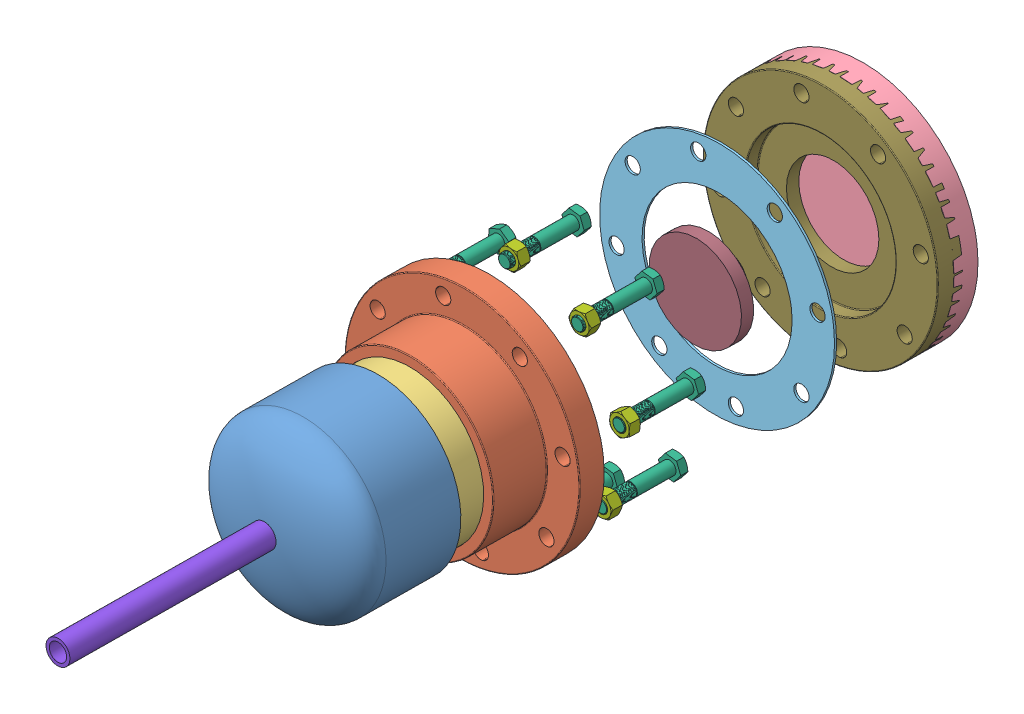
SolidWorks assembly Photogrametry_V4-PVC, configuration Default. Lengths in mm.
Overall size (408.7 414.98 1168.21).
29 component instances, 13 part files, 35 mates.
Components (placement in the parent):
- 8in PVC Cap-1: 8in PVC Cap [4881K523] at (-2621.5848 1342.0566 1037.7149) x (0.006396 0.016238 0.999848) z (-0.99998 0.000109 0.006395) size (216.92 247.14 247.14)
- 8in PVC Flange-1: 8in PVC Flange [4881K224] at (-2623.693 1336.7047 708.1733) x (0.979757 0.199965 -0.009515) z (0.006396 0.016238 0.999848) size (342.9 342.9 115.89)
- 8in PVC Pipe-1: 8in PVC Pipe [48855K43] at (-2622.9517 1338.5865 824.0432) x (0.99998 -0.000109 -0.006395) z (0.006396 0.016238 0.999848) size (219.07 219.07 203.2)
- 8in PVC Flange Closed-1: 8in PVC Flange Closed [4881K973] at (-2627.2283 1327.7296 155.5372) x (0.979757 0.199965 -0.009515) z (0.006396 0.016238 0.999848) size (342.9 342.9 36.51) (hidden)
- 8in Buna-N Gasket-1: 8in Buna-N Gasket [8516T54] at (-2625.8814 1331.149 366.0854) x (0.979757 0.199965 -0.009515) z (0.006396 0.016238 0.999848) size (342.9 342.9 3.17)
- BOLT 3-4in x 4in-1: BOLT 3-4in x 4in [92198A390] at (-2478.1489 1364.8686 603.567) x (0.006396 0.016238 0.999848) z (-0.923711 -0.382898 0.012128) size (114.21 33 28.57)
- BOLT 3-4in x 4in-2: BOLT 3-4in x 4in [92198A390] at (-2542.0965 1459.4699 600.4986) x (0.006396 0.016238 0.999848) z (-0.923711 -0.382898 0.012128) size (114.21 33 28.57)
- BOLT 3-4in x 4in-3: BOLT 3-4in x 4in [92198A390] at (-2499.8414 1252.7986 608.1398) x (0.006396 0.016238 0.999848) z (-0.923711 -0.382898 0.012128) size (114.21 33 28.57)
- BOLT 3-4in x 4in-4: BOLT 3-4in x 4in [92198A390] at (-2594.5008 1188.8228 606.2427) x (0.006396 0.016238 0.999848) z (-0.923711 -0.382898 0.012128) size (114.21 33 28.57)
- BOLT 3-4in x 4in-5: BOLT 3-4in x 4in [92198A390] at (-2748.8091 1417.4005 610.5319) x (0.006396 0.016238 0.999848) z (0.4222 -0.906423 0.01202) size (114.21 33 28.57)
- BOLT 3-4in x 4in-6: BOLT 3-4in x 4in [92198A390] at (-2654.2581 1481.1012 595.4899) x (0.006396 0.016238 0.999848) z (-0.923711 -0.382898 0.012128) size (114.21 33 28.57)
- BOLT 3-4in x 4in-9: BOLT 3-4in x 4in [92198A390] at (-2770.5384 1305.2371 609.3615) x (0.006396 0.016238 0.999848) z (-0.525994 0.850424 -0.010446) size (114.21 33 28.57)
- BOLT 3-4in x 4in-10: BOLT 3-4in x 4in [92198A390] at (-2706.607 1210.5947 609.8972) x (0.006396 0.016238 0.999848) z (-0.923711 -0.382898 0.012128) size (114.21 33 28.57)
- NUT 3-4in-2: NUT 3-4in [92676A510] at (-2477.0129 1365.6938 651.8097) x (0.999988 -0.000941 -0.004773) z (0.004802 0.034121 0.999406) size (28.57 33 20.12)
- NUT 3-4in-3: NUT 3-4in [92676A510] at (-2594.1923 1189.6059 654.4589) x (0.776919 0.629418 -0.015192) z (0.006396 0.016238 0.999848) size (28.57 33 20.12)
- NUT 3-4in-4: NUT 3-4in [92676A510] at (-2706.3607 1211.22 648.3989) x (0.776919 0.629418 -0.015192) z (0.006396 0.016238 0.999848) size (28.57 33 20.12)
- NUT 3-4in-5: NUT 3-4in [92676A510] at (-2499.5329 1253.5816 656.356) x (0.776919 0.629418 -0.015192) z (0.006396 0.016238 0.999848) size (28.57 33 20.12)
- NUT 3-4in-6: NUT 3-4in [92676A510] at (-2770.2861 1305.8775 648.7923) x (0.476506 0.879001 -0.017324) z (0.006396 0.016238 0.999848) size (28.57 33 20.12)
- NUT 3-4in-7: NUT 3-4in [92676A510] at (-2748.512 1418.1547 656.9726) x (-0.898727 0.438507 -0.001372) z (0.006396 0.016238 0.999848) size (28.57 33 20.12)
- NUT 3-4in-8: NUT 3-4in [92676A510] at (-2653.9915 1481.778 637.1682) x (0.923711 0.382898 -0.012128) z (0.006396 0.016238 0.999848) size (28.57 33 20.12)
- NUT 3-4in-9: NUT 3-4in [92676A510] at (-2541.8056 1460.2083 645.9637) x (0.827746 0.560918 -0.014405) z (0.006396 0.016238 0.999848) size (28.57 33 20.12)
- 5233K730_MASTERKLEER PVC TUBING-1: 5233K730_MASTERKLEER PVC TUBING [5233K73] at (-2620.6119 1344.5265 1189.7985) x (-0.006396 -0.016238 -0.999848) z (0.99998 -0.000109 -0.006395) size (304.8 34.92 34.92)
- camera case V3-1: camera case V3 [Default] at (-2623.6189 1336.8928 719.7548) x (-0.999819 -0.017794 0.006685) z (-0.006396 -0.016238 -0.999848) size (192 192 92)
- A7 III + FE 28-70 v4-1: A7 III + FE 28-70 v4 [Default] at (-2612.5666 1298.9736 748.4389) x (-0.999962 0 -0.008727) z (-0.000076 0.999962 0.008726) size (139.07 134.7 103.31)
  - A7 III + FE 28-70 v4.step-1: A7 III + FE 28-70 v4.step [Default] at origin size (139.07 134.7 103.31)
    - Sony A7 III.step-1: Sony A7 III.step [Default] at origin size (139.07 74.69 103.31)
    - Sony FE 28-70 mm f_3.5-5.6 OSS.step-1: Sony FE 28-70 mm f_3.5-5.6 OSS.step [Default] at (13.5 -93.5 40) size (72.5 83 72.5)
- 8in PVC Flange Closed - Dome Hole-1: 8in PVC Flange Closed - Dome Hole [4881K973] at (-2627.0814 1328.1025 178.499) x (0.979757 0.199965 -0.009515) z (0.006396 0.016238 0.999848) size (342.9 342.9 36.51)
- Custom Dome_v2.2-1: Custom Dome_v2.2 [Default] at (-2625.6652 1331.6979 399.8847) x (-0.924601 -0.380744 0.012098) z (0.380882 -0.924538 0.012578) size (135 55 135)
Mates (geometry in assembly coordinates):
- Coincident3: coincident anti-aligned: circle of 8in PVC Flange-1; circle of 8in PVC Pipe-1
- Concentric1: concentric anti-aligned: circle of 8in PVC Cap-1; circle of 8in PVC Pipe-1
- Concentric3: concentric anti-aligned: circle of 8in PVC Flange-1; circle of 8in Buna-N Gasket-1
- Concentric4: concentric aligned: circle of 8in PVC Flange Closed-1; circle of 8in Buna-N Gasket-1
- Concentric5: concentric aligned: circle of 8in PVC Flange Closed-1; circle of BOLT 3-4in x 4in-1
- Concentric16: concentric aligned: circle of 8in PVC Flange Closed-1; circle of BOLT 3-4in x 4in-2
- Concentric17: concentric aligned: circle of 8in PVC Flange Closed-1; circle of BOLT 3-4in x 4in-6
- Concentric18: concentric aligned: circle of 8in PVC Flange Closed-1; circle of BOLT 3-4in x 4in-5
- Concentric19: concentric aligned: circle of 8in PVC Flange Closed-1; circle of BOLT 3-4in x 4in-3
- Concentric20: concentric aligned: circle of 8in PVC Flange Closed-1; circle of BOLT 3-4in x 4in-4
- Concentric21: concentric aligned: circle of 8in PVC Flange Closed-1; circle of BOLT 3-4in x 4in-9
- Concentric22: concentric aligned: circle of 8in PVC Flange Closed-1; circle of BOLT 3-4in x 4in-10
- Concentric23: concentric aligned: circle of 8in PVC Flange Closed-1; circle of 8in Buna-N Gasket-1
- Concentric24: concentric aligned: circle of 8in PVC Flange-1; circle of 8in Buna-N Gasket-1
- Tangent2: tangent: curve of BOLT 3-4in x 4in-1; circle of NUT 3-4in-2
- Concentric26: concentric aligned: circle of BOLT 3-4in x 4in-4; circle of NUT 3-4in-3
- Concentric27: concentric aligned: circle of BOLT 3-4in x 4in-10; circle of NUT 3-4in-4
- Concentric28: concentric aligned: circle of BOLT 3-4in x 4in-3; circle of NUT 3-4in-5
- Concentric29: concentric aligned: circle of BOLT 3-4in x 4in-2; circle of NUT 3-4in-9
- Concentric30: concentric aligned: circle of BOLT 3-4in x 4in-6; circle of NUT 3-4in-8
- Concentric31: concentric aligned: circle of BOLT 3-4in x 4in-9; circle of NUT 3-4in-6
- Concentric32: concentric aligned: circle of BOLT 3-4in x 4in-5; circle of NUT 3-4in-7
- Coincident9: coincident anti-aligned: circle of 8in PVC Cap-1; circle of 5233K730_MASTERKLEER PVC TUBING-1
- Concentric33: concentric anti-aligned: circle of 8in PVC Pipe-1; circle of camera case V3-1
- Lock1: lock: unknown of camera case V3-1; unknown of A7 III + FE 28-70 v4-1/A7 III + FE 28-70 v4.step-1/Sony A7 III.step-1
- Concentric34: concentric anti-aligned: circle of 8in Buna-N Gasket-1; circle of 8in PVC Flange Closed - Dome Hole-1
- Concentric35: concentric aligned: circle of 8in Buna-N Gasket-1; circle of 8in PVC Flange Closed - Dome Hole-1
- Concentric36: concentric aligned: circle of 8in PVC Flange Closed - Dome Hole-1; circle of Custom Dome_v2.2-1
- Lock2: lock: unknown of BOLT 3-4in x 4in-5; unknown of NUT 3-4in-7
- Lock4: lock: unknown of BOLT 3-4in x 4in-2; unknown of NUT 3-4in-9
- Lock5: lock: unknown of BOLT 3-4in x 4in-1; unknown of NUT 3-4in-2
- Lock6: lock: unknown of BOLT 3-4in x 4in-3; unknown of NUT 3-4in-5
- Lock7: lock: unknown of BOLT 3-4in x 4in-4; unknown of NUT 3-4in-3
- Lock8: lock: unknown of BOLT 3-4in x 4in-10; unknown of NUT 3-4in-4
- Lock9: lock: unknown of BOLT 3-4in x 4in-6; unknown of NUT 3-4in-8
